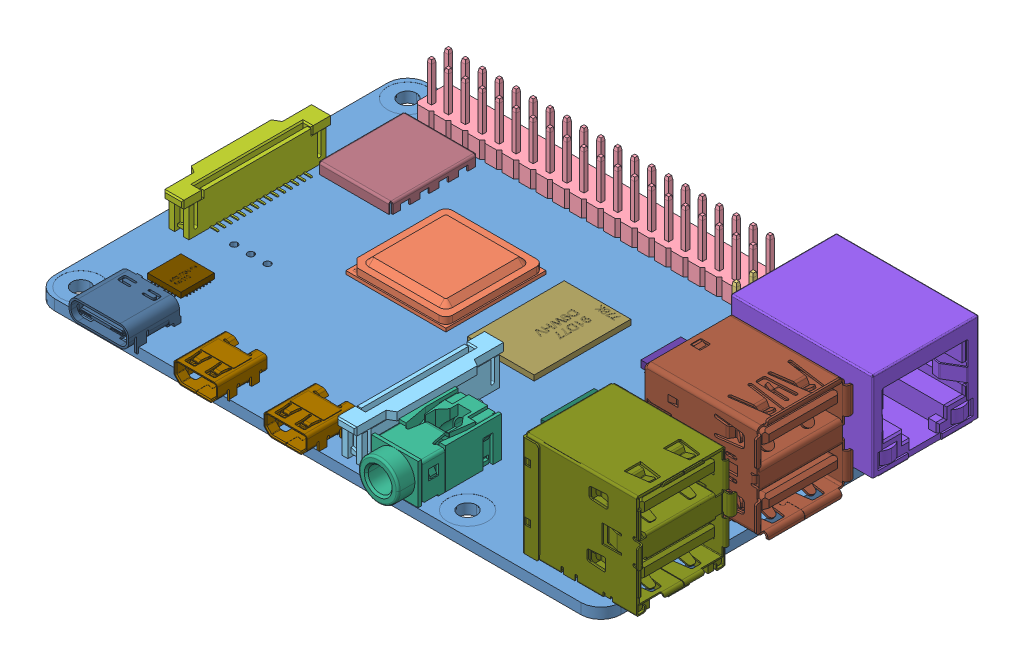
SolidWorks assembly rpi4b, configuration 默认. Lengths in mm.
Overall size (89 19.92 58.4).
20 component instances, 18 part files, 0 mates.
Components (placement in the parent):
- rpi4b(2)^rpi4b-1: rpi4b(2)^rpi4b [默认] at (-6.5308 1.9261 23.3348) size (89 19.92 58.4) (virtual)
  - PCB, RPi4ModelB^rpi4b(2)_rpi4b-1: PCB, RPi4ModelB^rpi4b(2)_rpi4b [默认] at origin size (85 1.6 56) (virtual)
  - Broadcom BCM2711B0 CPU, RPi4ModelB^rpi4b(2)_rpi4b-1: Broadcom BCM2711B0 CPU, RPi4ModelB^rpi4b(2)_rpi4b [默认] at (-13.25 0.8 -4.5) size (15 2.3 15) (virtual)
  - 2.54 mm DUPONT MALE PIN HEADER, POE, 2X2, RPi4ModelB^rpi4b(2)_rpi4b-1: 2.54 mm DUPONT MALE PIN HEADER, POE, 2X2, RPi4ModelB^rpi4b(2)_rpi4b [默认] at (19 0.8 -18.36) size (5.08 11.3 5.08) (virtual)
  - 2.54 mm DUPONT MALE PIN HEADER, IO, 2X20, RPi4ModelB^rpi4b(2)_rpi4b-1: 2.54 mm DUPONT MALE PIN HEADER, IO, 2X20, RPi4ModelB^rpi4b(2)_rpi4b [默认] at (-10 0.8 -24.5) size (50.8 11.3 5.08) (virtual)
  - Camera Connector, RPi4ModelB^rpi4b(2)_rpi4b-1: Camera Connector, RPi4ModelB^rpi4b(2)_rpi4b [默认] at (4 0.8 16.5) x (0 0 -1) z (1 0 0) size (22.4 5.68 5.07) (virtual)
  - Microphone Plug, RPi4ModelB^rpi4b(2)_rpi4b-1: Microphone Plug, RPi4ModelB^rpi4b(2)_rpi4b [默认] at (11.5 0.8 21.65) size (7.23 7.55 15) (virtual)
  - Display Connector, RPi4ModelB^rpi4b(2)_rpi4b-1: Display Connector, RPi4ModelB^rpi4b(2)_rpi4b [默认] at (-38.5 0.8 0) x (0 0 1) z (-1 0 0) size (22.4 5.68 5.07) (virtual)
  - Gigabit Ethernet Port, RPi4ModelB^rpi4b(2)_rpi4b-1: Gigabit Ethernet Port, RPi4ModelB^rpi4b(2)_rpi4b [默认] at (45.5 7.55 -17.75) x (0 0 -1) z (1 0 0) size (16.33 17.24 21.6) (virtual)
  - Female Micro HDMI Connector, RPi4ModelB^rpi4b(2)_rpi4b-1: Female Micro HDMI Connector, RPi4ModelB^rpi4b(2)_rpi4b [默认] at (-3 0.8 27.3875) size (6.5 3.51 7.5) (virtual)
  - Female Micro HDMI Connector, RPi4ModelB^rpi4b(2)_rpi4b-2: Female Micro HDMI Connector, RPi4ModelB^rpi4b(2)_rpi4b [默认] at (-16.5 0.8 27.3875) size (6.5 3.51 7.5) (virtual)
  - Female USB Type C Connector, RPi4ModelB^rpi4b(2)_rpi4b-1: Female USB Type C Connector, RPi4ModelB^rpi4b(2)_rpi4b [默认] at (-31.3 0.8 26.5419) size (8.94 3.96 7.9) (virtual)
  - 2X USB3.0 PORTS, RPi4ModelB^rpi4b(2)_rpi4b-1: 2X USB3.0 PORTS, RPi4ModelB^rpi4b(2)_rpi4b [默认] at (37.07 0.8 1) size (17.48 19.42 15.69) (virtual)
  - 91D77 D9WHV 778K, 4 GB LPDDR4 SDRAM, RPi4ModelB^rpi4b(2)_rpi4b-1: 91D77 D9WHV 778K, 4 GB LPDDR4 SDRAM, RPi4ModelB^rpi4b(2)_rpi4b [默认] at (2.25 0.8 -4.5) size (10 0.8 14.5) (virtual)
  - Cypress CYW43455 Wireless Module Cover, RPi4ModelB^rpi4b(2)_rpi4b-1: Cypress CYW43455 Wireless Module Cover, RPi4ModelB^rpi4b(2)_rpi4b [默认] at (-30.5 0.8 -14.5) size (11 1.6 13) (virtual)
  - SD Card Slot, RPi4ModelB^rpi4b(2)_rpi4b-1: SD Card Slot, RPi4ModelB^rpi4b(2)_rpi4b [默认] at (-35.3 -0.8 0) x (0 0 -1) z (-1 0 0) size (11.95 1.45 11.4) (virtual)
  - VIA VL805 PCIe USB 3.0 controller, RPi4ModelB^rpi4b(2)_rpi4b-1: VIA VL805 PCIe USB 3.0 controller, RPi4ModelB^rpi4b(2)_rpi4b [默认] at (17.5 0.8 4) size (8.8 0.8 8.8) (virtual)
  - 2X USB2.0 PORTS, RPi4ModelB^rpi4b(2)_rpi4b-1: 2X USB2.0 PORTS, RPi4ModelB^rpi4b(2)_rpi4b [默认] at (37.065 0.65 19) size (17.87 19.17 15.35) (virtual)
  - Broadcom BCM54213PE Gigabit Ethernet Transceiver, RPi4ModelB^rpi4b(2)_rpi4b-1: Broadcom BCM54213PE Gigabit Ethernet Transceiver, RPi4ModelB^rpi4b(2)_rpi4b [默认] at (16.5 0.8 -10) size (6.8 1 6.8) (virtual)
  - MxL7704 Universal PMIC, RPi4ModelB^rpi4b(2)_rpi4b-1: MxL7704 Universal PMIC, RPi4ModelB^rpi4b(2)_rpi4b [默认] at (-32.5 0.8 16) size (5.4 0.8 5.4) (virtual)
